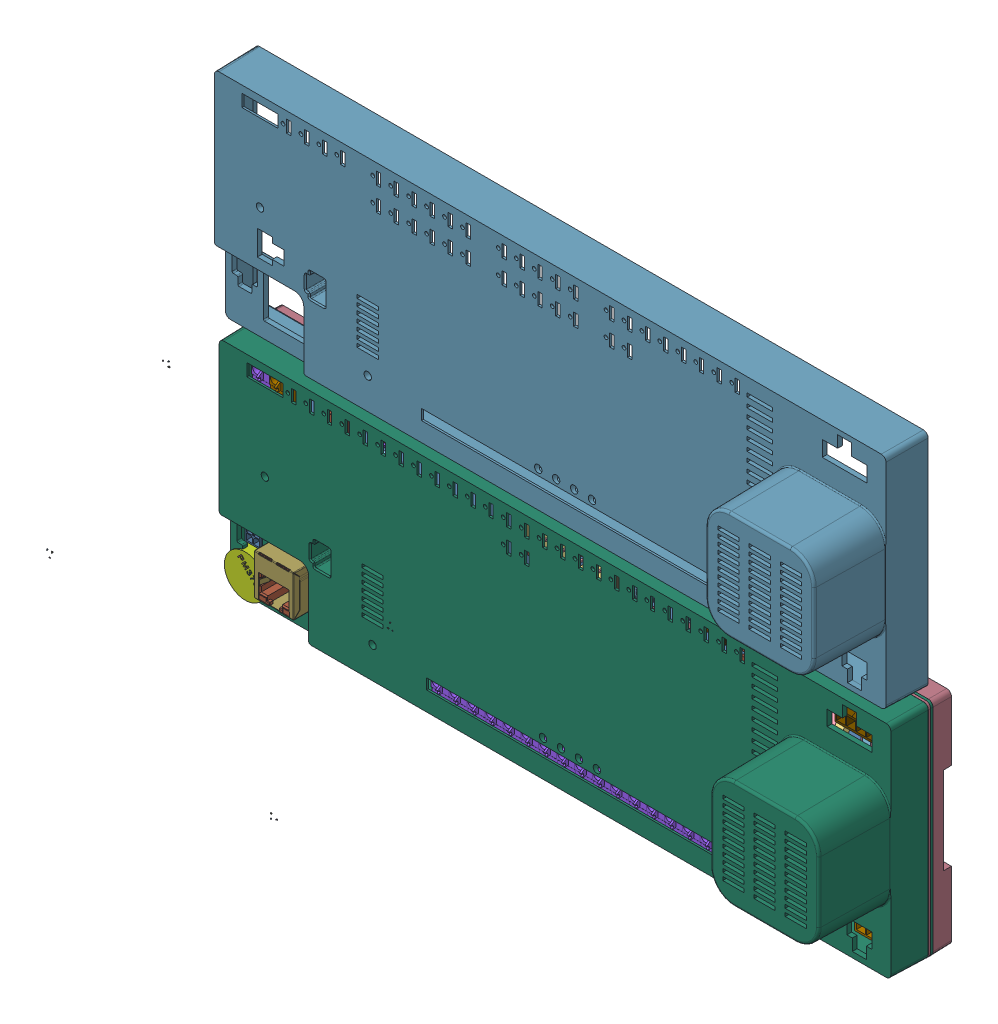
SolidWorks assembly _SC944D, configuration Default. Lengths in mm. (continued)
Components (placement in the parent): (continued)
- U11-1: U11 [Default] at origin size (3 3 1.35)
  - User_Library-SOT23-5-1-1: User_Library-SOT23-5-1 [Default] at (30.6387 50.3237 0) x (-1 0 0) z (0 0 1) size (3 3 1.35)
- U12-1: U12 [Default] at origin size (6.4 5.1 1.1)
  - User_Library-TSSOP-14_5_1x4_4-1: User_Library-TSSOP-14_5_1x4_4 [Default] at (241.0459 70.9689 0.6152) x (1 0 0) z (0 -1 0) size (6.4 1.1 5.1)
    - User_Library-TSSOP-14_5.1x4.4_pin_TSSOP_tssop_1-1: User_Library-TSSOP-14_5.1x4.4_pin_TSSOP_tssop_1 [Default] at (2.25 0 0.65) x (0 0 -1) z (1 0 0) size (0.25 0.65 0.95)
    - User_Library-TSSOP-14_5.1x4.4_pin_TSSOP_tssop_1-2: User_Library-TSSOP-14_5.1x4.4_pin_TSSOP_tssop_1 [Default] at (2.25 0 0) x (0 0 -1) z (1 0 0) size (0.25 0.65 0.95)
    - User_Library-TSSOP-14_5.1x4.4_pin_TSSOP_tssop_1-3: User_Library-TSSOP-14_5.1x4.4_pin_TSSOP_tssop_1 [Default] at (-2.25 0 1.95) x (0 0 1) z (-1 0 0) size (0.25 0.65 0.95)
    - User_Library-TSSOP-14_5.1x4.4_pin_TSSOP_tssop_1-4: User_Library-TSSOP-14_5.1x4.4_pin_TSSOP_tssop_1 [Default] at (2.25 0 1.3) x (0 0 -1) z (1 0 0) size (0.25 0.65 0.95)
    - User_Library-TSSOP-14_5.1x4.4_pin_TSSOP_tssop_1-5: User_Library-TSSOP-14_5.1x4.4_pin_TSSOP_tssop_1 [Default] at (-2.25 0 0.65) x (0 0 1) z (-1 0 0) size (0.25 0.65 0.95)
    - User_Library-TSSOP-14_5.1x4.4_pin_TSSOP_tssop_1-6: User_Library-TSSOP-14_5.1x4.4_pin_TSSOP_tssop_1 [Default] at (-2.25 0 -0.65) x (0 0 1) z (-1 0 0) size (0.25 0.65 0.95)
    - User_Library-TSSOP-14_5.1x4.4_pin_TSSOP_tssop_1-7: User_Library-TSSOP-14_5.1x4.4_pin_TSSOP_tssop_1 [Default] at (-2.25 0 -1.95) x (0 0 1) z (-1 0 0) size (0.25 0.65 0.95)
    - User_Library-TSSOP-14_5.1x4.4_pin_TSSOP_tssop_1-8: User_Library-TSSOP-14_5.1x4.4_pin_TSSOP_tssop_1 [Default] at (2.25 0 -1.3) x (0 0 -1) z (1 0 0) size (0.25 0.65 0.95)
    - User_Library-TSSOP-14_5.1x4.4_body_TSSOP_TSSOP_5.1x4.5_1-1: User_Library-TSSOP-14_5.1x4.4_body_TSSOP_TSSOP_5.1x4.5_1 [Default] at origin size (4.5 1 5.1)
    - User_Library-TSSOP-14_5.1x4.4_pin_TSSOP_tssop_1-9: User_Library-TSSOP-14_5.1x4.4_pin_TSSOP_tssop_1 [Default] at (2.25 0 -0.65) x (0 0 -1) z (1 0 0) size (0.25 0.65 0.95)
    - User_Library-TSSOP-14_5.1x4.4_pin_TSSOP_tssop_1-10: User_Library-TSSOP-14_5.1x4.4_pin_TSSOP_tssop_1 [Default] at (-2.25 0 -1.3) x (0 0 1) z (-1 0 0) size (0.25 0.65 0.95)
    - User_Library-TSSOP-14_5.1x4.4_pin_TSSOP_tssop_1-11: User_Library-TSSOP-14_5.1x4.4_pin_TSSOP_tssop_1 [Default] at (-2.25 0 0) x (0 0 1) z (-1 0 0) size (0.25 0.65 0.95)
    - User_Library-TSSOP-14_5.1x4.4_pin_TSSOP_tssop_1-12: User_Library-TSSOP-14_5.1x4.4_pin_TSSOP_tssop_1 [Default] at (-2.25 0 1.3) x (0 0 1) z (-1 0 0) size (0.25 0.65 0.95)
    - User_Library-TSSOP-14_5.1x4.4_pin_TSSOP_tssop_1-13: User_Library-TSSOP-14_5.1x4.4_pin_TSSOP_tssop_1 [Default] at (2.25 0 1.95) x (0 0 -1) z (1 0 0) size (0.25 0.65 0.95)
    - User_Library-TSSOP-14_5.1x4.4_pin_TSSOP_tssop_1-14: User_Library-TSSOP-14_5.1x4.4_pin_TSSOP_tssop_1 [Default] at (2.25 0 -1.95) x (0 0 -1) z (1 0 0) size (0.25 0.65 0.95)
- U13-1: U13 [Default] at origin size (9 9 1.48)
  - User_Library-LQFP48-7x7-0_50-1: User_Library-LQFP48-7x7-0_50 [Default] at (37.465 13.335 0.7652) x (0 -1 0) z (-1 0 0) size (9 1.48 9)
- U14-1: U14 [Default] at origin size (9.19 5.08 4.7)
  - SOIC_pin_2-1: SOIC_pin_2 [Default] at (91.765 48.4474 1) x (0 -1 0) z (-1 0 0) size (0.4 1.1 1.1)
  - SOIC_pin_2-2: SOIC_pin_2 [Default] at (94.7588 43.3774 1) x (0 1 0) z (1 0 0) size (0.4 1.1 1.1)
  - SOIC_pin_2-3: SOIC_pin_2 [Default] at (94.7588 40.8374 1) x (0 1 0) z (1 0 0) size (0.4 1.1 1.1)
  - SOIC_pin_2-4: SOIC_pin_2 [Default] at (91.765 50.9874 1) x (0 -1 0) z (-1 0 0) size (0.4 1.1 1.1)
  - 1175074120-1: 1175074120 [Default] at (89.9357 45.9124 0) size (0.41 5.08 4.5)
    - Extruded-1: Extruded [Default] at origin size (0.41 5.08 4.5)
  - 1175073984-1: 1175073984 [Default] at (93.2536 45.9123 0) size (7.05 5.08 4.6)
    - Extruded_1-1: Extruded_1 [Default] at origin size (7.05 5.08 4.6)
  - 1173467200-1: 1173467200 [Default] at (91.3487 47.8173 4.6) x (0 -1 0) z (0 0 1) size (0.4 0.4 0.1)
    - Cylinder_1-1: Cylinder_1 [Default] at origin size (0.4 0.4 0.1)
- U15-1: U15 [Default] at origin size (9.19 5.08 4.7)
  - SOIC_pin_2-1: SOIC_pin_2 [Default] at (91.765 54.7974 1) x (0 -1 0) z (-1 0 0) size (0.4 1.1 1.1)
  - SOIC_pin_2-2: SOIC_pin_2 [Default] at (94.7588 49.7274 1) x (0 1 0) z (1 0 0) size (0.4 1.1 1.1)
  - SOIC_pin_2-3: SOIC_pin_2 [Default] at (94.7588 47.1874 1) x (0 1 0) z (1 0 0) size (0.4 1.1 1.1)
  - SOIC_pin_2-4: SOIC_pin_2 [Default] at (91.765 57.3374 1) x (0 -1 0) z (-1 0 0) size (0.4 1.1 1.1)
  - 1175074120-1: 1175074120 [Default] at (89.9357 52.2624 0) size (0.41 5.08 4.5)
    - Extruded-1: Extruded [Default] at origin size (0.41 5.08 4.5)
  - 1175073984-1: 1175073984 [Default] at (93.2536 52.2623 0) size (7.05 5.08 4.6)
    - Extruded_1-1: Extruded_1 [Default] at origin size (7.05 5.08 4.6)
  - 1173467200-1: 1173467200 [Default] at (91.3487 54.1673 4.6) x (0 -1 0) z (0 0 1) size (0.4 0.4 0.1)
    - Cylinder_1-1: Cylinder_1 [Default] at origin size (0.4 0.4 0.1)
- U16-1: U16 [Default] at origin size (7 6.5 1.65)
  - SW3dPS-SOT-223-1-1: SW3dPS-SOT-223-1 [Default] at (188.7604 53.785 0.75) x (1 0 0) z (0 -1 0) size (7 1.65 6.5)
- U17-1: U17 [Default] at origin size (6.5 7 1.65)
  - SW3dPS-SOT-223-1-1: SW3dPS-SOT-223-1 [Default] at (77.1284 38.7088 0.75) x (0 1 0) z (1 0 0) size (7 1.65 6.5)
- U19-1: U19 [Default] at origin size (3.1 2.3 0.86)
  - SW3dPS-VSSOP8-1: SW3dPS-VSSOP8 [Default] at (5.3351 23.495 0.45) x (-1 0 0) z (0 1 0) size (3.1 0.85 2.3)
  - 1173467328-1: 1173467328 [Default] at (5.9339 22.7951 0.76) x (0 1 0) z (0 0 1) size (0.4 0.4 0.08)
    - Cylinder_6-1: Cylinder_6 [Default] at origin size (0.4 0.4 0.08)
- U22-1: U22 [Default] at origin size (9.8 19.5 14.1)
  - 1175074392-1: 1175074392 [Default] at (0.3174 43.8151 -1.6) size (0.5 0.5 1.6)
    - Extruded_2-1: Extruded_2 [Default] at origin size (0.5 0.5 1.6)
  - 1175074392-2: 1175074392 [Default] at (0.3174 41.2751 -1.6) size (0.5 0.5 1.6)
    - Extruded_2-1: Extruded_2 [Default] at origin size (0.5 0.5 1.6)
  - 1175074392-3: 1175074392 [Default] at (0.3174 38.7351 -1.6) size (0.5 0.5 1.6)
    - Extruded_2-1: Extruded_2 [Default] at origin size (0.5 0.5 1.6)
  - 1175074392-4: 1175074392 [Default] at (0.3174 31.1151 -1.6) size (0.5 0.5 1.6)
    - Extruded_2-1: Extruded_2 [Default] at origin size (0.5 0.5 1.6)
  - 1175074392-5: 1175074392 [Default] at (0.3174 28.5751 -1.6) size (0.5 0.5 1.6)
    - Extruded_2-1: Extruded_2 [Default] at origin size (0.5 0.5 1.6)
  - 1175074664-1: 1175074664 [Default] at (2.8175 36.425 0) size (9.8 19.5 12.5)
    - Extruded_21-1: Extruded_21 [Default] at origin size (9.8 19.5 12.5)
- U25-1: U25 [Default] at origin size (9.19 5.08 4.7)
  - SOIC_pin_2-1: SOIC_pin_2 [Default] at (17.5614 56.0338 1) x (0 -1 0) z (-1 0 0) size (0.4 1.1 1.1)
  - SOIC_pin_2-2: SOIC_pin_2 [Default] at (20.5552 50.9637 1) x (0 1 0) z (1 0 0) size (0.4 1.1 1.1)
  - SOIC_pin_2-3: SOIC_pin_2 [Default] at (20.5552 48.4238 1) x (0 1 0) z (1 0 0) size (0.4 1.1 1.1)
  - SOIC_pin_2-4: SOIC_pin_2 [Default] at (17.5614 58.5737 1) x (0 -1 0) z (-1 0 0) size (0.4 1.1 1.1)
  - 1175074120-1: 1175074120 [Default] at (15.7322 53.4987 0) size (0.41 5.08 4.5)
    - Extruded-1: Extruded [Default] at origin size (0.41 5.08 4.5)
  - 1175073984-1: 1175073984 [Default] at (19.05 53.4987 0) size (7.05 5.08 4.6)
    - Extruded_1-1: Extruded_1 [Default] at origin size (7.05 5.08 4.6)
  - 1173467200-1: 1173467200 [Default] at (17.1451 55.4037 4.6) x (0 -1 0) z (0 0 1) size (0.4 0.4 0.1)
    - Cylinder_1-1: Cylinder_1 [Default] at origin size (0.4 0.4 0.1)
- VR1-1: VR1 [Default] at origin size (37.34 26.17 33.9)
  - WE-VD_14_mm-1: WE-VD_14_mm [Default] at (233.0058 7.4853 8) x (0.309017 -0.951057 0) z (0.672498 0.218508 0.707107) size (16.5 6.44 41.5)
- R160-1: R160 [Default] at origin size (1.6 0.8 0.55)
  - RESC1608X84N-1: RESC1608X84N [Default] at (40.7988 25.7175 0) x (1 0 0) z (0 -1 0) size (1.6 0.55 0.8)
- R161-1: R161 [Default] at origin size (0.8 1.6 0.55)
  - RESC1608X84N-1: RESC1608X84N [Default] at (210.8201 40.1319 0) x (0 -1 0) z (-1 0 0) size (1.6 0.55 0.8)
- D67-1: D67 [Default] at origin size (5.3 3.6 1.11)
  - 1175071672-1: 1175071672 [Default] at (234.839 79.883 0) size (5.3 3.6 1.1)
    - Extruded_12-1: Extruded_12 [Default] at origin size (5.3 3.6 1.1)
  - 1175071536-1: 1175071536 [Default] at (233.3023 79.883 1.1) size (0.79 3.56 0.01)
    - Extruded_13-1: Extruded_13 [Default] at origin size (0.79 3.56 0.01)
- R64-1: R64 [Default] at origin size (1.6 0.8 0.55)
  - RESC1608X84N-1: RESC1608X84N [Default] at (231.1045 73.4061 0) x (1 0 0) z (0 -1 0) size (1.6 0.55 0.8)
- D52-1: D52 [Default] at origin size (82.13 96.14 23.48)
  - SW3dPS-transistor_SOT233-1: SW3dPS-transistor_SOT233 [Default] at (78.6512 93.2681 -21.9) x (1 0 0) z (0 -1 0) size (2.9 1.1 1.6)
  - SW3dPS-transistor_SOT233_1-1: SW3dPS-transistor_SOT233_1 [Default] at (0.0787 0.0933 -0.0219) x (1 0 0) z (0 -1 0) size (2.18 2.18 2.18)
  - SW3dPS-transistor_SOT233_2-1: SW3dPS-transistor_SOT233_2 [Default] at (0.0001 0.0001 0) x (1 0 0) z (0 -1 0) size (2.18 2.18 2.18)
  - SW3dPS-transistor_SOT233_3-1: SW3dPS-transistor_SOT233_3 [Default] x (1 0 0) z (0 -1 0) size (2.18 2.18 2.18)
- T13-1: T13 [Default] at origin size (6.73 10.1 2.41)
  - DPAK_TO-252AA_RGB8421504-1: DPAK_TO-252AA_RGB8421504 [Default] at (128.2698 27.3977 0.0428) x (-1 0 0) z (0 1 0) size (6.73 2.41 10.1)
- R89-1: R89 [Default] at origin size (1.6 0.8 0.55)
  - RESC1608X84N-1: RESC1608X84N [Default] at (103.5049 40.64 0) x (-1 0 0) z (0 1 0) size (1.6 0.55 0.8)
- C139-1: C139 [Default] at origin size (1.6 0.8 0.9)
  - User_Library-CAPC1608X09-1: User_Library-CAPC1608X09 [Default] at (111.7601 60.8331 0) x (1 0 0) z (0 0 1) size (1.6 0.8 0.9)
- C140-1: C140 [Default] at origin size (0.8 1.6 0.9)
  - User_Library-CAPC1608X09-1: User_Library-CAPC1608X09 [Default] at (106.4259 61.9761 0) x (0 1 0) z (0 0 1) size (1.6 0.8 0.9)
- C141-1: C141 [Default] at origin size (1.6 0.8 0.9)
  - User_Library-CAPC1608X09-1: User_Library-CAPC1608X09 [Default] at (144.9069 60.0709 0) x (-1 0 0) z (0 0 1) size (1.6 0.8 0.9)
- C142-1: C142 [Default] at origin size (0.8 1.6 0.9)
  - User_Library-CAPC1608X09-1: User_Library-CAPC1608X09 [Default] at (193.1671 70.3262 0) x (0 -1 0) z (0 0 1) size (1.6 0.8 0.9)
- D66-1: D66 [Default] at origin size (42.29 37.97 23.48)
  - SW3dPS-transistor_SOT233-1: SW3dPS-transistor_SOT233 [Default] at (38.8238 35.0972 -21.9) x (-1 0 0) z (0 1 0) size (2.9 1.1 1.6)
  - SW3dPS-transistor_SOT233_1-1: SW3dPS-transistor_SOT233_1 [Default] at (0.0388 0.0351 -0.0219) x (-1 0 0) z (0 1 0) size (2.18 2.18 2.18)
  - SW3dPS-transistor_SOT233_2-1: SW3dPS-transistor_SOT233_2 [Default] at (0 0 0) x (-1 0 0) z (0 1 0) size (2.18 2.18 2.18)
  - SW3dPS-transistor_SOT233_3-1: SW3dPS-transistor_SOT233_3 [Default] x (-1 0 0) z (0 1 0) size (2.18 2.18 2.18)
- D68-1: D68 [Default] at origin size (83.31 137.12 23.48)
  - SW3dPS-transistor_SOT233-1: SW3dPS-transistor_SOT233 [Default] at (80.4362 133.6422 -21.9) x (0 1 0) z (1 0 0) size (2.9 1.1 1.6)
  - SW3dPS-transistor_SOT233_1-1: SW3dPS-transistor_SOT233_1 [Default] at (0.0804 0.1336 -0.0219) x (0 1 0) z (1 0 0) size (2.18 2.18 2.18)
  - SW3dPS-transistor_SOT233_2-1: SW3dPS-transistor_SOT233_2 [Default] at (0.0001 0.0001 0) x (0 1 0) z (1 0 0) size (2.18 2.18 2.18)
  - SW3dPS-transistor_SOT233_3-1: SW3dPS-transistor_SOT233_3 [Default] x (0 1 0) z (1 0 0) size (2.18 2.18 2.18)
- D69-1: D69 [Default] at origin size (177.58 20.41 23.48)
  - SW3dPS-transistor_SOT233-1: SW3dPS-transistor_SOT233 [Default] at (174.7068 -16.9292 -21.9) x (0 -1 0) z (-1 0 0) size (2.9 1.1 1.6)
  - SW3dPS-transistor_SOT233_1-1: SW3dPS-transistor_SOT233_1 [Default] at (0.1747 -0.0169 -0.0219) x (0 -1 0) z (-1 0 0) size (2.18 2.18 2.18)
  - SW3dPS-transistor_SOT233_2-1: SW3dPS-transistor_SOT233_2 [Default] at (0.0002 0 0) x (0 -1 0) z (-1 0 0) size (2.18 2.18 2.18)
  - SW3dPS-transistor_SOT233_3-1: SW3dPS-transistor_SOT233_3 [Default] x (0 -1 0) z (-1 0 0) size (2.18 2.18 2.18)
- D70-1: D70 [Default] at origin size (127.67 46.48 23.48)
  - SW3dPS-transistor_SOT233-1: SW3dPS-transistor_SOT233 [Default] at (124.2948 43.6062 -21.9) x (-1 0 0) z (0 1 0) size (2.9 1.1 1.6)
  - SW3dPS-transistor_SOT233_1-1: SW3dPS-transistor_SOT233_1 [Default] at (0.1243 0.0436 -0.0219) x (-1 0 0) z (0 1 0) size (2.18 2.18 2.18)
  - SW3dPS-transistor_SOT233_2-1: SW3dPS-transistor_SOT233_2 [Default] at (0.0001 0 0) x (-1 0 0) z (0 1 0) size (2.18 2.18 2.18)
  - SW3dPS-transistor_SOT233_3-1: SW3dPS-transistor_SOT233_3 [Default] x (-1 0 0) z (0 1 0) size (2.18 2.18 2.18)
- L43-1: L43 [Default] at origin size (0.8 1.6 0.9)
  - User_Library-CAPC1608X09-1: User_Library-CAPC1608X09 [Default] at (114.1731 65.0239 0) x (0 -1 0) z (0 0 1) size (1.6 0.8 0.9)
- L44-1: L44 [Default] at origin size (0.8 1.6 0.9)
  - User_Library-CAPC1608X09-1: User_Library-CAPC1608X09 [Default] at (109.9821 65.0239 0) x (0 -1 0) z (0 0 1) size (1.6 0.8 0.9)
- L45-1: L45 [Default] at origin size (1.6 0.8 0.9)
  - User_Library-CAPC1608X09-1: User_Library-CAPC1608X09 [Default] at (143.0021 65.0241 0) x (1 0 0) z (0 0 1) size (1.6 0.8 0.9)
- L46-1: L46 [Default] at origin size (1.6 0.8 0.9)
  - User_Library-CAPC1608X09-1: User_Library-CAPC1608X09 [Default] at (194.3101 72.7711 0) x (1 0 0) z (0 0 1) size (1.6 0.8 0.9)
- R172-1: R172 [Default] at origin size (0.8 1.6 0.55)
  - RESC1608X84N-1: RESC1608X84N [Default] at (112.3951 65.0239 0) x (0 -1 0) z (-1 0 0) size (1.6 0.55 0.8)
- R173-1: R173 [Default] at origin size (1.6 0.8 0.55)
  - RESC1608X84N-1: RESC1608X84N [Default] at (111.7599 62.6109 0) x (-1 0 0) z (0 1 0) size (1.6 0.55 0.8)
- R174-1: R174 [Default] at origin size (0.8 1.6 0.55)
  - RESC1608X84N-1: RESC1608X84N [Default] at (108.204 65.0239 0) x (0 -1 0) z (-1 0 0) size (1.6 0.55 0.8)
- R180-1: R180 [Default] at origin size (0.8 1.6 0.55)
  - RESC1608X84N-1: RESC1608X84N [Default] at (108.204 61.9759 0) x (0 -1 0) z (-1 0 0) size (1.6 0.55 0.8)
- R181-1: R181 [Default] at origin size (0.8 1.6 0.55)
  - RESC1608X84N-1: RESC1608X84N [Default] at (143.637 62.4841 0) x (0 1 0) z (1 0 0) size (1.6 0.55 0.8)
- R182-1: R182 [Default] at origin size (0.8 1.6 0.55)
  - RESC1608X84N-1: RESC1608X84N [Default] at (145.415 62.4839 0) x (0 -1 0) z (-1 0 0) size (1.6 0.55 0.8)
- R183-1: R183 [Default] at origin size (0.8 1.6 0.55)
  - RESC1608X84N-1: RESC1608X84N [Default] at (197.0087 70.3263 0) x (0 1 0) z (1 0 0) size (1.6 0.55 0.8)
- R187-1: R187 [Default] at origin size (0.8 1.6 0.55)
  - RESC1608X84N-1: RESC1608X84N [Default] at (194.9451 70.3262 0) x (0 -1 0) z (-1 0 0) size (1.6 0.55 0.8)
- R178-1: R178 [Default] at origin size (1.6 0.8 0.55)
  - RESC1608X84N-1: RESC1608X84N [Default] at (203.0412 71.12 0) x (-1 0 0) z (0 1 0) size (1.6 0.55 0.8)
- R188-1: R188 [Default] at origin size (0.8 1.6 0.55)
  - RESC1608X84N-1: RESC1608X84N [Default] at (51.7525 44.7674 0) x (0 -1 0) z (-1 0 0) size (1.6 0.55 0.8)
- R192-1: R192 [Default] at origin size (1.6 0.8 0.55)
  - RESC1608X84N-1: RESC1608X84N [Default] at (3.6512 51.2762 0) x (-1 0 0) z (0 1 0) size (1.6 0.55 0.8)
- R200-1: R200 [Default] at origin size (1.6 0.8 0.55)
  - RESC1608X84N-1: RESC1608X84N [Default] at (7.1438 51.2763 0) x (1 0 0) z (0 -1 0) size (1.6 0.55 0.8)
- R105-1: R105 [Default] at origin size (1.6 0.8 0.55)
  - RESC1608X84N-1: RESC1608X84N [Default] at (48.4188 43.3388 0) x (1 0 0) z (0 -1 0) size (1.6 0.55 0.8)
- C120-1: C120 [Default] at origin size (2 1.25 1)
  - User_Library-CAPC2013X10-1: User_Library-CAPC2013X10 [Default] at (44.2914 38.5763 0) x (1 0 0) z (0 0 1) size (2 1.25 1)
- R36-1: R36 [Default] at origin size (0.8 1.6 0.55)
  - RESC1608X84N-1: RESC1608X84N [Default] at (83.1849 35.4013 0) x (0 1 0) z (1 0 0) size (1.6 0.55 0.8)
- R86-1: R86 [Default] at origin size (0.8 1.6 0.55)
  - RESC1608X84N-1: RESC1608X84N [Default] at (100.7109 45.3391 0) x (0 1 0) z (1 0 0) size (1.6 0.55 0.8)
- R96-1: R96 [Default] at origin size (1.6 0.8 0.55)
  - RESC1608X84N-1: RESC1608X84N [Default] at (78.6131 29.3371 0) x (1 0 0) z (0 -1 0) size (1.6 0.55 0.8)
- R98-1: R98 [Default] at origin size (1.6 0.8 0.55)
  - RESC1608X84N-1: RESC1608X84N [Default] at (73.7871 29.972 0) x (1 0 0) z (0 -1 0) size (1.6 0.55 0.8)
- R99-1: R99 [Default] at origin size (1.6 0.8 0.55)
  - RESC1608X84N-1: RESC1608X84N [Default] at (78.6131 30.9881 0) x (1 0 0) z (0 -1 0) size (1.6 0.55 0.8)
- C12-1: C12 [Default] at origin size (1.6 0.8 0.9)
  - User_Library-CAPC1608X09-1: User_Library-CAPC1608X09 [Default] at (76.9621 24.5111 0) x (1 0 0) z (0 0 1) size (1.6 0.8 0.9)
- C73-1: C73 [Default] at origin size (1.6 0.8 0.9)
  - User_Library-CAPC1608X09-1: User_Library-CAPC1608X09 [Default] at (76.9621 22.7331 0) x (1 0 0) z (0 0 1) size (1.6 0.8 0.9)
- R101-1: R101 [Default] at origin size (1.6 0.8 0.55)
  - RESC1608X84N-1: RESC1608X84N [Default] at (78.7399 27.5589 0) x (-1 0 0) z (0 1 0) size (1.6 0.55 0.8)
- F6-1: F6 [Default] at origin size (5.69 7.27 15.9)
  - mf-rx012_250-1: mf-rx012_250 [Default] at (128.2701 14.351 6.7) x (0.000349 0 1) z (-1 0 0.000349) size (15.9 7.27 5.69)
- F7-1: F7 [Default] at origin size (5.69 7.27 15.9)
  - mf-rx012_250-1: mf-rx012_250 [Default] at (137.5411 14.224 6.7) x (0.000349 0 1) z (-1 0 0.000349) size (15.9 7.27 5.69)
- F8-1: F8 [Default] at origin size (5.69 7.27 15.9)
  - mf-rx012_250-1: mf-rx012_250 [Default] at (146.3041 14.224 6.7) x (0.000349 0 1) z (-1 0 0.000349) size (15.9 7.27 5.69)
- F9-1: F9 [Default] at origin size (5.69 7.27 15.9)
  - mf-rx012_250-1: mf-rx012_250 [Default] at (155.0671 14.224 6.7) x (0.000349 0 1) z (-1 0 0.000349) size (15.9 7.27 5.69)
- U18-1: U18 [Default] at origin size (2.3 2.1 1)
  - User_Library-sot353-1: User_Library-sot353 [Default] at (192.793 66.768 0) x (0 -1 0) z (0 0 1) size (2.1 2.3 1)
- U20-1: U20 [Default] at origin size (2.3 2.1 1)
  - User_Library-sot353-1: User_Library-sot353 [Default] at (199.8733 73.626 0) x (0 -1 0) z (0 0 1) size (2.1 2.3 1)
- Free-Models-1: Free-Models [Default] at origin size (285.98 194 57.6)
  - Coque_inférieure_commune_BA+BP_v3.0_(Valla)-1: Coque_inférieure_commune_BA+BP_v3.0_(Valla) [Default] at (135.865 -7.64 0) x (1 0 0) z (0 -1 0) size (285.8 11.8 94)
  - top_Coque_supérieure_BP_(944)_v2.0_(Valla)_RGB8421504-1: top_Coque_supérieure_BP_(944)_v2.0_(Valla)_RGB8421504 [Default] at (135.865 186.36 0) x (1 0 0) z (0 -1 0) size (285.8 47.6 94)
  - 000coque_boitier_principal_(Valla_Stéréo_2)-1: 000coque_boitier_principal_(Valla_Stéréo_2) [Default] at (135.92 86.38 -2) x (1 0 0) z (0 -1 0) size (285.93 47.6 94)
  - Coque_inférieure_commune_BA+BP_v3.0_(Valla)-2: Coque_inférieure_commune_BA+BP_v3.0_(Valla) [Default] at (135.92 -7.62 0) x (1 0 0) z (0 -1 0) size (285.8 11.8 94)
